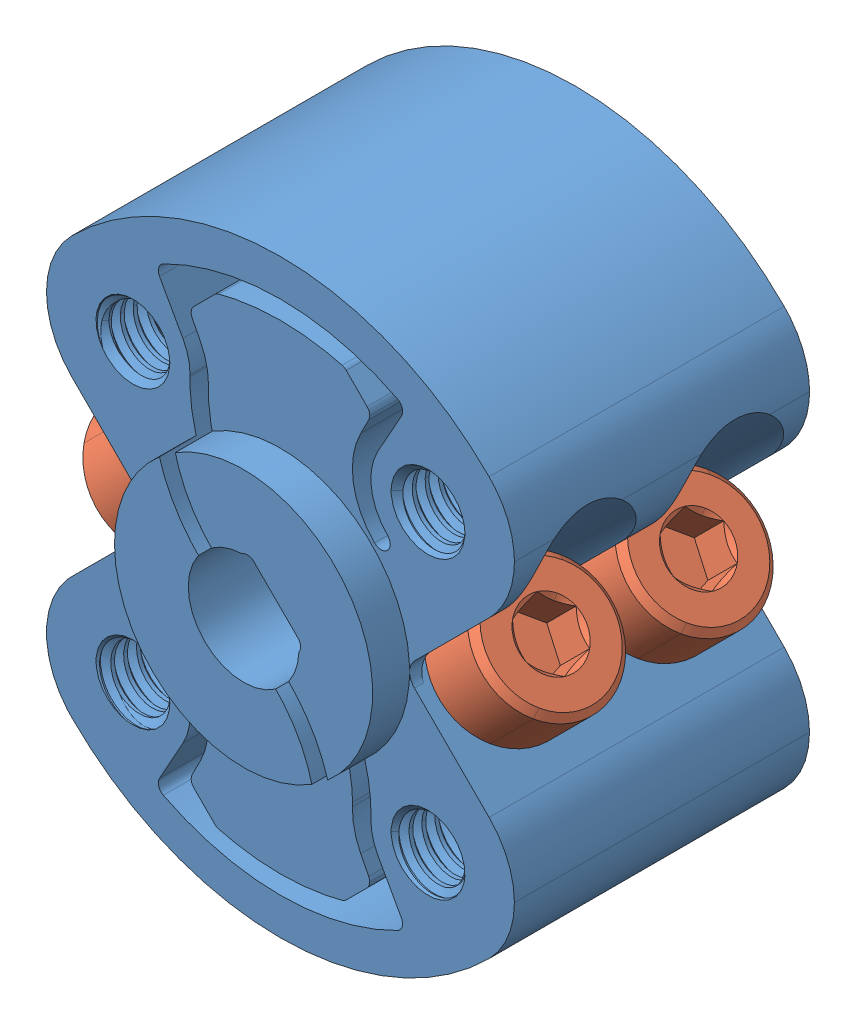
SolidWorks assembly 1312-0016-1006 Assembly, configuration Default. Lengths in mm.
Overall size (28.36 32 18.95).
6 component instances, 2 part files, 0 mates.
Components (placement in the parent):
- 1312-0016-1006 Assembly.STEP-1: 1312-0016-1006 Assembly.STEP [Default] at origin size (28.36 32 18.95)
  - 1312-0016-1006.STEP-1: 1312-0016-1006.STEP [Default] at (-23.4637 -17.2124 31.7239) size (25.38 32 18)
  - 2800-0004-0014_90128A207.STEP-1: 2800-0004-0014_90128A207.STEP [Default] at (-25.5166 -28.3312 27.7239) x (0.5 -0.5 0.707107) z (-0.707107 -0.707107 0) size (7 7 18.01)
  - 2800-0004-0014_90128A207.STEP-2: 2800-0004-0014_90128A207.STEP [Default] at (-25.5166 -28.3312 19.7239) x (0.5 -0.5 0.707107) z (-0.707107 -0.707107 0) size (7 7 18.01)
  - 2800-0004-0014_90128A207.STEP-3: 2800-0004-0014_90128A207.STEP [Default] at (-21.4109 -6.0937 27.7239) x (-0.5 0.5 0.707107) z (0.707107 0.707107 0) size (7 7 18.01)
  - 2800-0004-0014_90128A207.STEP-4: 2800-0004-0014_90128A207.STEP [Default] at (-21.4109 -6.0937 19.7239) x (-0.5 0.5 0.707107) z (0.707107 0.707107 0) size (7 7 18.01)
